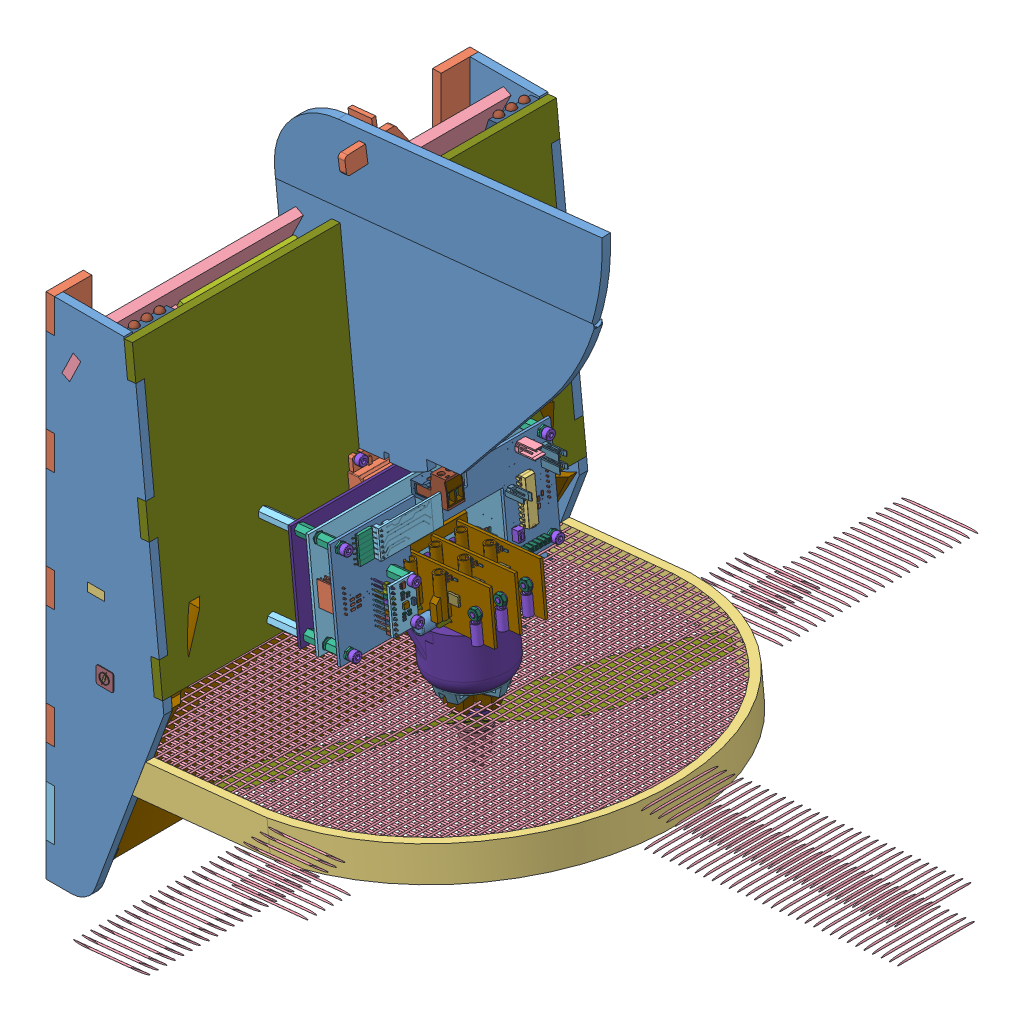
SolidWorks assembly AssTotale, configuration Défaut. Lengths in mm. (continued)
Components (placement in the parent): (continued)
- AssStructSimu-1: AssStructSimu [Défaut] at (-75.9431 -10.8604 24.5323) size (253.25 324.59 251.6) (continued)
  - AssCarte-1: AssCarte [Défaut] at (-42.8534 32.2132 302.028) x (-0.101852 0.9948 0) z (0.9948 0.101852 0) size (67.15 130.57 98.45) (continued)
    - carte_onduleur_v4-1: carte_onduleur_v4 [Défaut] at (-25.7639 0.8332 112.9379) size (66.52 130.57 82.34) (continued)
      - CON_IO1-1: CON_IO1 [Défaut] at (-11.3 12.1 0.803) x (0 -1 0) z (0 0 1) size (16.74 30.7 57.5) (continued)
        - Open CASCADE STEP translator 6.8 1.3.1-1: Open CASCADE STEP translator 6.8 1.3.1 [Défaut] at origin size (16.74 30.7 57.5) (continued)
          - Body_1_2-1: Body_1_2 [Défaut] at (-3 -15 8) x (0 -1 0) z (-1 0 0) size (30.7 57.5 16.74) (continued)
            - 57-1: 57 [Défaut] at (-15.3 2.7 -0.803) x (0 -1 0) z (0 0 -1) size (10.36 15.24 6.14) (continued)
              - =_[0_1_1_47]-1: =_[0_1_1_47] [Défaut] at origin size (10.36 15.24 6.14) (continued)
                - 55-1: 55 [Défaut] at (1.8 -1.2 3) x (1 0 0) z (0 1 0) size (10.36 6.14 15.24) (continued)
                  - 54-2: 54 [Défaut] at (0 0 -7.62) size (10.36 6.14 7.62) (continued)
                    - 52-2: 52 [Défaut] at (0 0 -2.54) size (10.36 6.14 2.54) (continued)
                      - 48-1: 48 [Défaut] at origin size (8.4 2.54 2.54)
                      - 49-1: 49 [Défaut] at (-0.0461 1.2682 1.27) x (0 0 -1) z (0.999998 -0.002105 0) size (1.95 5.07 7.58)
                    - 52-3: 52 [Défaut] at (0 0 -5.08) size (10.36 6.14 2.54)
                      - 48-1: 48 [Défaut] at origin size (8.4 2.54 2.54)
                      - 49-1: 49 [Défaut] at (-0.0461 1.2682 1.27) x (0 0 -1) z (0.999998 -0.002105 0) size (1.95 5.07 7.58)
            - 59-1: 59 [Défaut] at (-26.5 31 0.803) x (0 -1 0) z (0 0 1) size (2.34 1.04 0.5)
              - =_[0_1_1_42]-1: =_[0_1_1_42] [Défaut] at origin size (2.34 1.04 0.5)
                - 43-1: 43 [Défaut] at origin size (2.29 1.04 0.43)
                - 44-1: 44 [Défaut] at (0.3048 0 0) x (-1 0 0) z (0 0 1) size (0.51 1.02 0.5)
                - 45-1: 45 [Défaut] at origin size (0.51 1.02 0.5)
            - 61-1: 61 [Défaut] at (-21.6 17.8 0.803) x (-1 0 0) z (0 0 1) size (2.34 1.04 0.5)
              - =_[0_1_1_42]-1: =_[0_1_1_42] [Défaut] at origin size (2.34 1.04 0.5)
                - 43-1: 43 [Défaut] at origin size (2.29 1.04 0.43)
                - 44-1: 44 [Défaut] at (0.3048 0 0) x (-1 0 0) z (0 0 1) size (0.51 1.02 0.5)
                - 45-1: 45 [Défaut] at origin size (0.51 1.02 0.5)
            - 64-1: 64 [Défaut] at (-3.3 17.6 0.803) x (0 -1 0) z (0 0 1) size (8.01 8 14.24)
              - =_[0_1_1_56]-1: =_[0_1_1_56] [Défaut] at origin size (8.01 8 14.24)
                - 62-1: 62 [Défaut] at (1.8 0 0) x (1 0 0) z (0 -1 0) size (8.01 14.24 8)
      - CON_IO2-1: CON_IO2 [Défaut] at (-11.3 -2.7 0.803) x (0 -1 0) z (0 0 1) size (16.74 30.7 57.5)
        - Open CASCADE STEP translator 6.8 1.4.1-1: Open CASCADE STEP translator 6.8 1.4.1 [Défaut] at origin size (16.74 30.7 57.5)
          - Body_1_2-1: Body_1_2 [Défaut] at (-3 -15 8) x (0 -1 0) z (-1 0 0) size (30.7 57.5 16.74)
            - 1-1: 1 [Défaut] at origin size (30 50 1.61)
            - 10-1: 10 [Défaut] at (-14.395 31.0465 0.803) x (-1 0 0) z (0 0 1) size (5.59 6.35 1.11)
              - =_[0_1_1_4]-1: =_[0_1_1_4] [Défaut] at origin size (5.59 6.35 1.11)
                - 11-1: 11 [Défaut] at (2 3.3 0) x (-1 0 0) z (0 0 1) size (5.59 6.35 1.11)
                  - =_[0_1_1_3]_2-1: =_[0_1_1_3]_2 [Défaut] at origin size (0.44 0.55 0.36)
                  - =_[0_1_1_4]_2-1: =_[0_1_1_4]_2 [Défaut] at origin size (5.59 4.15 0.36)
                  - =_[0_1_1_5]_2-1: =_[0_1_1_5]_2 [Défaut] at origin size (5.35 6.1 1.1)
                  - =_[0_1_1_6]-1: =_[0_1_1_6] [Défaut] at origin size (0.44 0.55 0.36)
                  - =_[0_1_1_7]-1: =_[0_1_1_7] [Défaut] at origin size (0.44 0.55 0.36)
                  - =_[0_1_1_8]-1: =_[0_1_1_8] [Défaut] at origin size (0.44 0.55 0.36)
            - 13-1: 13 [Défaut] at (-12.62 16.6 -0.803) x (-1 0 0) z (0 0 -1) size (5.59 6.35 1.11)
              - =_[0_1_1_13]-1: =_[0_1_1_13] [Défaut] at origin size (5.59 6.35 1.11)
                - 11-1: 11 [Défaut] at (2 3.3 0) x (-1 0 0) z (0 0 1) size (5.59 6.35 1.11)
                  - =_[0_1_1_3]_2-1: =_[0_1_1_3]_2 [Défaut] at origin size (0.44 0.55 0.36)
                  - =_[0_1_1_4]_2-1: =_[0_1_1_4]_2 [Défaut] at origin size (5.59 4.15 0.36)
                  - =_[0_1_1_5]_2-1: =_[0_1_1_5]_2 [Défaut] at origin size (5.35 6.1 1.1)
                  - =_[0_1_1_6]-1: =_[0_1_1_6] [Défaut] at origin size (0.44 0.55 0.36)
                  - =_[0_1_1_7]-1: =_[0_1_1_7] [Défaut] at origin size (0.44 0.55 0.36)
                  - =_[0_1_1_8]-1: =_[0_1_1_8] [Défaut] at origin size (0.44 0.55 0.36)
            - 16-1: 16 [Défaut] at (-4.2 24.2 0.803) x (-1 0 0) z (0 0 1) size (12.8 0.5 13)
              - =_[0_1_1_15]-1: =_[0_1_1_15] [Défaut] at origin size (12.8 0.5 13)
                - 17-1: 17 [Défaut] at (2.7 0 0) x (1 0 0) z (0 -1 0) size (12.8 13 0.5)
            - 19-1: 19 [Défaut] at (-4.1 6.8 0.803) x (-1 0 0) z (0 0 1) size (12.8 0.5 13)
              - =_[0_1_1_18]-1: =_[0_1_1_18] [Défaut] at origin size (12.8 0.5 13)
                - 17-1: 17 [Défaut] at (2.7 0 0) x (1 0 0) z (0 -1 0) size (12.8 13 0.5)
            - 24-1: 24 [Défaut] at (-8.1 16.5 -0.803) x (0 1 0) z (0 0 -1) size (7.75 5.13 1.17)
              - =_[0_1_1_20]-1: =_[0_1_1_20] [Défaut] at origin size (7.75 5.13 1.17)
                - 20-1: 20 [Défaut] at origin size (7.59 5.13 1.07)
                - 21-1: 21 [Défaut] at (-14.478 0 0) x (-1 0 0) z (0 0 1) size (0.76 5.08 1.17)
                - 22-1: 22 [Défaut] at origin size (0.76 5.08 1.17)
            - 35-1: 35 [Défaut] at (-25.3 25.5 0.803) x (0 -1 0) z (0 0 1) size (6.05 5.2 1.7)
              - =_[0_1_1_25]-1: =_[0_1_1_25] [Défaut] at origin size (6.05 5.2 1.7)
                - 25-1: 25 [Défaut] at origin size (4.3 5.2 1.53)
                - 26-1: 26 [Défaut] at origin size (0.88 0.51 1.06)
                - 27-1: 27 [Défaut] at origin size (0.88 0.51 1.06)
                - 28-1: 28 [Défaut] at origin size (0.88 0.51 1.06)
                - 29-1: 29 [Défaut] at origin size (0.88 0.51 1.06)
                - 30-1: 30 [Défaut] at (11.6 -5.08 0) x (-1 0 0) z (0 0 1) size (0.87 0.51 1.06)
                - 31-1: 31 [Défaut] at (11.6 -2.54 0) x (-1 0 0) z (0 0 1) size (0.87 0.51 1.06)
                - 32-1: 32 [Défaut] at (11.6 0 0) x (-1 0 0) z (0 0 1) size (0.87 0.51 1.06)
                - 33-1: 33 [Défaut] at (11.6 2.54 0) x (-1 0 0) z (0 0 1) size (0.87 0.51 1.06)
            - 40-1: 40 [Défaut] at (-27.6 27.2 0.803) size (2.34 1.04 0.5)
              - =_[0_1_1_36]-1: =_[0_1_1_36] [Défaut] at origin size (2.34 1.04 0.5)
                - 36-1: 36 [Défaut] at origin size (2.29 1.04 0.43)
                - 37-1: 37 [Défaut] at (0.3048 0 0) x (-1 0 0) z (0 0 1) size (0.51 1.02 0.5)
                - 38-1: 38 [Défaut] at origin size (0.51 1.02 0.5)
            - 42-1: 42 [Défaut] at (-22.1 21.6 0.803) x (0 1 0) z (0 0 1) size (2.34 1.04 0.5)
              - =_[0_1_1_36]-1: =_[0_1_1_36] [Défaut] at origin size (2.34 1.04 0.5)
                - 36-1: 36 [Défaut] at origin size (2.29 1.04 0.43)
                - 37-1: 37 [Défaut] at (0.3048 0 0) x (-1 0 0) z (0 0 1) size (0.51 1.02 0.5)
                - 38-1: 38 [Défaut] at origin size (0.51 1.02 0.5)
            - 47-1: 47 [Défaut] at (-14.7664 14.5 -0.803) x (-1 0 0) z (0 0 -1) size (2.34 1.04 0.5)
              - =_[0_1_1_42]-1: =_[0_1_1_42] [Défaut] at origin size (2.34 1.04 0.5)
                - 43-1: 43 [Défaut] at origin size (2.29 1.04 0.43)
                - 44-1: 44 [Défaut] at (0.3048 0 0) x (-1 0 0) z (0 0 1) size (0.51 1.02 0.5)
                - 45-1: 45 [Défaut] at origin size (0.51 1.02 0.5)
            - 57-1: 57 [Défaut] at (-15.3 2.7 -0.803) x (0 -1 0) z (0 0 -1) size (10.36 15.24 6.14)
              - =_[0_1_1_47]-1: =_[0_1_1_47] [Défaut] at origin size (10.36 15.24 6.14)
                - 55-1: 55 [Défaut] at (1.8 -1.2 3) x (1 0 0) z (0 1 0) size (10.36 6.14 15.24)
                  - 54-1: 54 [Défaut] at origin size (10.36 6.14 7.62)
                    - 52-1: 52 [Défaut] at origin size (10.36 6.14 2.54)
                      - 48-1: 48 [Défaut] at origin size (8.4 2.54 2.54)
                      - 49-1: 49 [Défaut] at (-0.0461 1.2682 1.27) x (0 0 -1) z (0.999998 -0.002105 0) size (1.95 5.07 7.58)
                    - 52-2: 52 [Défaut] at (0 0 -2.54) size (10.36 6.14 2.54)
                      - 48-1: 48 [Défaut] at origin size (8.4 2.54 2.54)
                      - 49-1: 49 [Défaut] at (-0.0461 1.2682 1.27) x (0 0 -1) z (0.999998 -0.002105 0) size (1.95 5.07 7.58)
                    - 52-3: 52 [Défaut] at (0 0 -5.08) size (10.36 6.14 2.54)
                      - 48-1: 48 [Défaut] at origin size (8.4 2.54 2.54)
                      - 49-1: 49 [Défaut] at (-0.0461 1.2682 1.27) x (0 0 -1) z (0.999998 -0.002105 0) size (1.95 5.07 7.58)
                  - 54-2: 54 [Défaut] at (0 0 -7.62) size (10.36 6.14 7.62)
                    - 52-1: 52 [Défaut] at origin size (10.36 6.14 2.54)
                      - 48-1: 48 [Défaut] at origin size (8.4 2.54 2.54)
                      - 49-1: 49 [Défaut] at (-0.0461 1.2682 1.27) x (0 0 -1) z (0.999998 -0.002105 0) size (1.95 5.07 7.58)
                    - 52-2: 52 [Défaut] at (0 0 -2.54) size (10.36 6.14 2.54)
                      - 48-1: 48 [Défaut] at origin size (8.4 2.54 2.54)
                      - 49-1: 49 [Défaut] at (-0.0461 1.2682 1.27) x (0 0 -1) z (0.999998 -0.002105 0) size (1.95 5.07 7.58)
                    - 52-3: 52 [Défaut] at (0 0 -5.08) size (10.36 6.14 2.54)
                      - 48-1: 48 [Défaut] at origin size (8.4 2.54 2.54)
                      - 49-1: 49 [Défaut] at (-0.0461 1.2682 1.27) x (0 0 -1) z (0.999998 -0.002105 0) size (1.95 5.07 7.58)
            - 59-1: 59 [Défaut] at (-26.5 31 0.803) x (0 -1 0) z (0 0 1) size (2.34 1.04 0.5)
              - =_[0_1_1_42]-1: =_[0_1_1_42] [Défaut] at origin size (2.34 1.04 0.5)
                - 43-1: 43 [Défaut] at origin size (2.29 1.04 0.43)
                - 44-1: 44 [Défaut] at (0.3048 0 0) x (-1 0 0) z (0 0 1) size (0.51 1.02 0.5)
                - 45-1: 45 [Défaut] at origin size (0.51 1.02 0.5)
            - 61-1: 61 [Défaut] at (-21.6 17.8 0.803) x (-1 0 0) z (0 0 1) size (2.34 1.04 0.5)
              - =_[0_1_1_42]-1: =_[0_1_1_42] [Défaut] at origin size (2.34 1.04 0.5)
                - 43-1: 43 [Défaut] at origin size (2.29 1.04 0.43)
                - 44-1: 44 [Défaut] at (0.3048 0 0) x (-1 0 0) z (0 0 1) size (0.51 1.02 0.5)
                - 45-1: 45 [Défaut] at origin size (0.51 1.02 0.5)
            - 64-1: 64 [Défaut] at (-3.3 17.6 0.803) x (0 -1 0) z (0 0 1) size (8.01 8 14.24)
              - =_[0_1_1_56]-1: =_[0_1_1_56] [Défaut] at origin size (8.01 8 14.24)
                - 62-1: 62 [Défaut] at (1.8 0 0) x (1 0 0) z (0 -1 0) size (8.01 14.24 8)
      - CON_IO3-1: CON_IO3 [Défaut] at (-11.3 -17.7 0.803) x (0 -1 0) z (0 0 1) size (16.74 30.7 57.5)
        - Open CASCADE STEP translator 6.8 1.5.1-1: Open CASCADE STEP translator 6.8 1.5.1 [Défaut] at origin size (16.74 30.7 57.5)
          - Body_1_2-1: Body_1_2 [Défaut] at (-3 -15 8) x (0 -1 0) z (-1 0 0) size (30.7 57.5 16.74)
            - 1-1: 1 [Défaut] at origin size (30 50 1.61)
            - 10-1: 10 [Défaut] at (-14.395 31.0465 0.803) x (-1 0 0) z (0 0 1) size (5.59 6.35 1.11)
              - =_[0_1_1_4]-1: =_[0_1_1_4] [Défaut] at origin size (5.59 6.35 1.11)
                - 11-1: 11 [Défaut] at (2 3.3 0) x (-1 0 0) z (0 0 1) size (5.59 6.35 1.11)
                  - =_[0_1_1_3]_2-1: =_[0_1_1_3]_2 [Défaut] at origin size (0.44 0.55 0.36)
                  - =_[0_1_1_4]_2-1: =_[0_1_1_4]_2 [Défaut] at origin size (5.59 4.15 0.36)
                  - =_[0_1_1_5]_2-1: =_[0_1_1_5]_2 [Défaut] at origin size (5.35 6.1 1.1)
                  - =_[0_1_1_6]-1: =_[0_1_1_6] [Défaut] at origin size (0.44 0.55 0.36)
                  - =_[0_1_1_7]-1: =_[0_1_1_7] [Défaut] at origin size (0.44 0.55 0.36)
                  - =_[0_1_1_8]-1: =_[0_1_1_8] [Défaut] at origin size (0.44 0.55 0.36)
            - 13-1: 13 [Défaut] at (-12.62 16.6 -0.803) x (-1 0 0) z (0 0 -1) size (5.59 6.35 1.11)
              - =_[0_1_1_13]-1: =_[0_1_1_13] [Défaut] at origin size (5.59 6.35 1.11)
                - 11-1: 11 [Défaut] at (2 3.3 0) x (-1 0 0) z (0 0 1) size (5.59 6.35 1.11)
                  - =_[0_1_1_3]_2-1: =_[0_1_1_3]_2 [Défaut] at origin size (0.44 0.55 0.36)
                  - =_[0_1_1_4]_2-1: =_[0_1_1_4]_2 [Défaut] at origin size (5.59 4.15 0.36)
                  - =_[0_1_1_5]_2-1: =_[0_1_1_5]_2 [Défaut] at origin size (5.35 6.1 1.1)
                  - =_[0_1_1_6]-1: =_[0_1_1_6] [Défaut] at origin size (0.44 0.55 0.36)
                  - =_[0_1_1_7]-1: =_[0_1_1_7] [Défaut] at origin size (0.44 0.55 0.36)
                  - =_[0_1_1_8]-1: =_[0_1_1_8] [Défaut] at origin size (0.44 0.55 0.36)
            - 16-1: 16 [Défaut] at (-4.2 24.2 0.803) x (-1 0 0) z (0 0 1) size (12.8 0.5 13)
              - =_[0_1_1_15]-1: =_[0_1_1_15] [Défaut] at origin size (12.8 0.5 13)
                - 17-1: 17 [Défaut] at (2.7 0 0) x (1 0 0) z (0 -1 0) size (12.8 13 0.5)
            - 19-1: 19 [Défaut] at (-4.1 6.8 0.803) x (-1 0 0) z (0 0 1) size (12.8 0.5 13)
              - =_[0_1_1_18]-1: =_[0_1_1_18] [Défaut] at origin size (12.8 0.5 13)
                - 17-1: 17 [Défaut] at (2.7 0 0) x (1 0 0) z (0 -1 0) size (12.8 13 0.5)
            - 24-1: 24 [Défaut] at (-8.1 16.5 -0.803) x (0 1 0) z (0 0 -1) size (7.75 5.13 1.17)
              - =_[0_1_1_20]-1: =_[0_1_1_20] [Défaut] at origin size (7.75 5.13 1.17)
                - 20-1: 20 [Défaut] at origin size (7.59 5.13 1.07)
                - 21-1: 21 [Défaut] at (-14.478 0 0) x (-1 0 0) z (0 0 1) size (0.76 5.08 1.17)
                - 22-1: 22 [Défaut] at origin size (0.76 5.08 1.17)
            - 35-1: 35 [Défaut] at (-25.3 25.5 0.803) x (0 -1 0) z (0 0 1) size (6.05 5.2 1.7)
              - =_[0_1_1_25]-1: =_[0_1_1_25] [Défaut] at origin size (6.05 5.2 1.7)
                - 25-1: 25 [Défaut] at origin size (4.3 5.2 1.53)
                - 26-1: 26 [Défaut] at origin size (0.88 0.51 1.06)
                - 27-1: 27 [Défaut] at origin size (0.88 0.51 1.06)
                - 28-1: 28 [Défaut] at origin size (0.88 0.51 1.06)
                - 29-1: 29 [Défaut] at origin size (0.88 0.51 1.06)
                - 30-1: 30 [Défaut] at (11.6 -5.08 0) x (-1 0 0) z (0 0 1) size (0.87 0.51 1.06)
                - 31-1: 31 [Défaut] at (11.6 -2.54 0) x (-1 0 0) z (0 0 1) size (0.87 0.51 1.06)
                - 32-1: 32 [Défaut] at (11.6 0 0) x (-1 0 0) z (0 0 1) size (0.87 0.51 1.06)
                - 33-1: 33 [Défaut] at (11.6 2.54 0) x (-1 0 0) z (0 0 1) size (0.87 0.51 1.06)
            - 40-1: 40 [Défaut] at (-27.6 27.2 0.803) size (2.34 1.04 0.5)
              - =_[0_1_1_36]-1: =_[0_1_1_36] [Défaut] at origin size (2.34 1.04 0.5)
                - 36-1: 36 [Défaut] at origin size (2.29 1.04 0.43)
                - 37-1: 37 [Défaut] at (0.3048 0 0) x (-1 0 0) z (0 0 1) size (0.51 1.02 0.5)
                - 38-1: 38 [Défaut] at origin size (0.51 1.02 0.5)
            - 42-1: 42 [Défaut] at (-22.1 21.6 0.803) x (0 1 0) z (0 0 1) size (2.34 1.04 0.5)
              - =_[0_1_1_36]-1: =_[0_1_1_36] [Défaut] at origin size (2.34 1.04 0.5)
                - 36-1: 36 [Défaut] at origin size (2.29 1.04 0.43)
                - 37-1: 37 [Défaut] at (0.3048 0 0) x (-1 0 0) z (0 0 1) size (0.51 1.02 0.5)
                - 38-1: 38 [Défaut] at origin size (0.51 1.02 0.5)
            - 47-1: 47 [Défaut] at (-14.7664 14.5 -0.803) x (-1 0 0) z (0 0 -1) size (2.34 1.04 0.5)
              - =_[0_1_1_42]-1: =_[0_1_1_42] [Défaut] at origin size (2.34 1.04 0.5)
                - 43-1: 43 [Défaut] at origin size (2.29 1.04 0.43)
                - 44-1: 44 [Défaut] at (0.3048 0 0) x (-1 0 0) z (0 0 1) size (0.51 1.02 0.5)
                - 45-1: 45 [Défaut] at origin size (0.51 1.02 0.5)
            - 57-1: 57 [Défaut] at (-15.3 2.7 -0.803) x (0 -1 0) z (0 0 -1) size (10.36 15.24 6.14)
              - =_[0_1_1_47]-1: =_[0_1_1_47] [Défaut] at origin size (10.36 15.24 6.14)
                - 55-1: 55 [Défaut] at (1.8 -1.2 3) x (1 0 0) z (0 1 0) size (10.36 6.14 15.24)
                  - 54-1: 54 [Défaut] at origin size (10.36 6.14 7.62)
                    - 52-1: 52 [Défaut] at origin size (10.36 6.14 2.54)
                      - 48-1: 48 [Défaut] at origin size (8.4 2.54 2.54)
                      - 49-1: 49 [Défaut] at (-0.0461 1.2682 1.27) x (0 0 -1) z (0.999998 -0.002105 0) size (1.95 5.07 7.58)
                    - 52-2: 52 [Défaut] at (0 0 -2.54) size (10.36 6.14 2.54)
                      - 48-1: 48 [Défaut] at origin size (8.4 2.54 2.54)
                      - 49-1: 49 [Défaut] at (-0.0461 1.2682 1.27) x (0 0 -1) z (0.999998 -0.002105 0) size (1.95 5.07 7.58)
                    - 52-3: 52 [Défaut] at (0 0 -5.08) size (10.36 6.14 2.54)
                      - 48-1: 48 [Défaut] at origin size (8.4 2.54 2.54)
                      - 49-1: 49 [Défaut] at (-0.0461 1.2682 1.27) x (0 0 -1) z (0.999998 -0.002105 0) size (1.95 5.07 7.58)
                  - 54-2: 54 [Défaut] at (0 0 -7.62) size (10.36 6.14 7.62)
                    - 52-1: 52 [Défaut] at origin size (10.36 6.14 2.54)
                      - 48-1: 48 [Défaut] at origin size (8.4 2.54 2.54)
                      - 49-1: 49 [Défaut] at (-0.0461 1.2682 1.27) x (0 0 -1) z (0.999998 -0.002105 0) size (1.95 5.07 7.58)
                    - 52-2: 52 [Défaut] at (0 0 -2.54) size (10.36 6.14 2.54)
                      - 48-1: 48 [Défaut] at origin size (8.4 2.54 2.54)
                      - 49-1: 49 [Défaut] at (-0.0461 1.2682 1.27) x (0 0 -1) z (0.999998 -0.002105 0) size (1.95 5.07 7.58)
                    - 52-3: 52 [Défaut] at (0 0 -5.08) size (10.36 6.14 2.54)
                      - 48-1: 48 [Défaut] at origin size (8.4 2.54 2.54)
                      - 49-1: 49 [Défaut] at (-0.0461 1.2682 1.27) x (0 0 -1) z (0.999998 -0.002105 0) size (1.95 5.07 7.58)
            - 59-1: 59 [Défaut] at (-26.5 31 0.803) x (0 -1 0) z (0 0 1) size (2.34 1.04 0.5)
              - =_[0_1_1_42]-1: =_[0_1_1_42] [Défaut] at origin size (2.34 1.04 0.5)
                - 43-1: 43 [Défaut] at origin size (2.29 1.04 0.43)
                - 44-1: 44 [Défaut] at (0.3048 0 0) x (-1 0 0) z (0 0 1) size (0.51 1.02 0.5)
                - 45-1: 45 [Défaut] at origin size (0.51 1.02 0.5)
            - 61-1: 61 [Défaut] at (-21.6 17.8 0.803) x (-1 0 0) z (0 0 1) size (2.34 1.04 0.5)
              - =_[0_1_1_42]-1: =_[0_1_1_42] [Défaut] at origin size (2.34 1.04 0.5)
                - 43-1: 43 [Défaut] at origin size (2.29 1.04 0.43)
                - 44-1: 44 [Défaut] at (0.3048 0 0) x (-1 0 0) z (0 0 1) size (0.51 1.02 0.5)
                - 45-1: 45 [Défaut] at origin size (0.51 1.02 0.5)
            - 64-1: 64 [Défaut] at (-3.3 17.6 0.803) x (0 -1 0) z (0 0 1) size (8.01 8 14.24)
              - =_[0_1_1_56]-1: =_[0_1_1_56] [Défaut] at origin size (8.01 8 14.24)
                - 62-1: 62 [Défaut] at (1.8 0 0) x (1 0 0) z (0 -1 0) size (8.01 14.24 8)
      - C1_1-1: C1_1 [Défaut] at (-20.6336 6.4 -0.803) x (1 0 0) z (0 0 -1) size (2.34 1.04 0.5)
        - Open CASCADE STEP translator 6.8 1.6.1-1: Open CASCADE STEP translator 6.8 1.6.1 [Défaut] at origin size (2.34 1.04 0.5)
          - Body_1-1: Body_1 [Défaut] at origin size (2.29 1.04 0.43)
          - Pin_1-1: Pin_1 [Défaut] at (0.3048 0 0) x (-1 0 0) z (0 0 1) size (0.51 1.02 0.5)
          - Pin_2-1: Pin_2 [Défaut] at origin size (0.51 1.02 0.5)
      - C1_2-1: C1_2 [Défaut] at (-24.2 6.4 -0.803) x (1 0 0) z (0 0 -1) size (2.34 1.04 0.5)
        - Open CASCADE STEP translator 6.8 1.6.1-1: Open CASCADE STEP translator 6.8 1.6.1 [Défaut] at origin size (2.34 1.04 0.5)
          - Body_1-1: Body_1 [Défaut] at origin size (2.29 1.04 0.43)
          - Pin_1-1: Pin_1 [Défaut] at (0.3048 0 0) x (-1 0 0) z (0 0 1) size (0.51 1.02 0.5)
          - Pin_2-1: Pin_2 [Défaut] at origin size (0.51 1.02 0.5)
      - C_F-1: C_F [Défaut] at (-16.2432 4.45 -0.803) x (0 -1 0) z (0 0 -1) size (2.34 1.04 0.5)
        - Open CASCADE STEP translator 6.8 1.6.1-1: Open CASCADE STEP translator 6.8 1.6.1 [Défaut] at origin size (2.34 1.04 0.5)
          - Body_1-1: Body_1 [Défaut] at origin size (2.29 1.04 0.43)
          - Pin_1-1: Pin_1 [Défaut] at (0.3048 0 0) x (-1 0 0) z (0 0 1) size (0.51 1.02 0.5)
          - Pin_2-1: Pin_2 [Défaut] at origin size (0.51 1.02 0.5)
      - D_LED_STATE1-1: D_LED_STATE1 [Défaut] at (-6.8906 -21.6 0.803) size (2.34 1.04 0.5)
        - Open CASCADE STEP translator 6.8 1.6.1-1: Open CASCADE STEP translator 6.8 1.6.1 [Défaut] at origin size (2.34 1.04 0.5)
          - Body_1-1: Body_1 [Défaut] at origin size (2.29 1.04 0.43)
          - Pin_1-1: Pin_1 [Défaut] at (0.3048 0 0) x (-1 0 0) z (0 0 1) size (0.51 1.02 0.5)
          - Pin_2-1: Pin_2 [Défaut] at origin size (0.51 1.02 0.5)
      - PICKIT-1: PICKIT [Défaut] at (-24.1 -30.5 0.803) size (15.24 5 14.3)
        - Open CASCADE STEP translator 6.8 1.10.1-1: Open CASCADE STEP translator 6.8 1.10.1 [Défaut] at origin size (15.24 5 14.3)
          - Body_1_2-1: Body_1_2 [Défaut] at (6.3 0 12) size (15.24 5 14.3)
      - C_DEC_CUR-1: C_DEC_CUR [Défaut] at (-8.9496 5.7572 -0.803) x (0 1 0) z (0 0 -1) size (2.34 1.04 0.5)
        - Open CASCADE STEP translator 6.8 1.6.1-1: Open CASCADE STEP translator 6.8 1.6.1 [Défaut] at origin size (2.34 1.04 0.5)
          - Body_1-1: Body_1 [Défaut] at origin size (2.29 1.04 0.43)
          - Pin_1-1: Pin_1 [Défaut] at (0.3048 0 0) x (-1 0 0) z (0 0 1) size (0.51 1.02 0.5)
          - Pin_2-1: Pin_2 [Défaut] at origin size (0.51 1.02 0.5)
      - R_F-1: R_F [Défaut] at (-14.65 4.4432 -0.803) x (0 -1 0) z (0 0 -1) size (2.34 1.04 0.5)
        - Open CASCADE STEP translator 6.8 1.12.1-1: Open CASCADE STEP translator 6.8 1.12.1 [Défaut] at origin size (2.34 1.04 0.5)
          - Body_1_3-1: Body_1_3 [Défaut] at origin size (2.29 1.04 0.43)
          - Pin_1_2-1: Pin_1_2 [Défaut] at (0.3048 0 0) x (-1 0 0) z (0 0 1) size (0.51 1.02 0.5)
          - Pin_2_2-1: Pin_2_2 [Défaut] at origin size (0.51 1.02 0.5)
      - R_GAIN1-1: R_GAIN1 [Défaut] at (-13.95 5.7568 -0.803) x (0 1 0) z (0 0 -1) size (2.34 1.04 0.5)
        - Open CASCADE STEP translator 6.8 1.12.1-1: Open CASCADE STEP translator 6.8 1.12.1 [Défaut] at origin size (2.34 1.04 0.5)
          - Body_1_3-1: Body_1_3 [Défaut] at origin size (2.29 1.04 0.43)
          - Pin_1_2-1: Pin_1_2 [Défaut] at (0.3048 0 0) x (-1 0 0) z (0 0 1) size (0.51 1.02 0.5)
          - Pin_2_2-1: Pin_2_2 [Défaut] at origin size (0.51 1.02 0.5)
      - R_GAIN2-1: R_GAIN2 [Défaut] at (-15.65 7.9176 -0.803) x (0 -1 0) z (0 0 -1) size (2.34 1.04 0.5)
        - Open CASCADE STEP translator 6.8 1.12.1-1: Open CASCADE STEP translator 6.8 1.12.1 [Défaut] at origin size (2.34 1.04 0.5)
          - Body_1_3-1: Body_1_3 [Défaut] at origin size (2.29 1.04 0.43)
          - Pin_1_2-1: Pin_1_2 [Défaut] at (0.3048 0 0) x (-1 0 0) z (0 0 1) size (0.51 1.02 0.5)
          - Pin_2_2-1: Pin_2_2 [Défaut] at origin size (0.51 1.02 0.5)
      - R_LED_STATE1-1: R_LED_STATE1 [Défaut] at (-6.9242 -19.9 0.803) size (2.34 1.04 0.5)
        - Open CASCADE STEP translator 6.8 1.12.1-1: Open CASCADE STEP translator 6.8 1.12.1 [Défaut] at origin size (2.34 1.04 0.5)
          - Body_1_3-1: Body_1_3 [Défaut] at origin size (2.29 1.04 0.43)
          - Pin_1_2-1: Pin_1_2 [Défaut] at (0.3048 0 0) x (-1 0 0) z (0 0 1) size (0.51 1.02 0.5)
          - Pin_2_2-1: Pin_2_2 [Défaut] at origin size (0.51 1.02 0.5)
      - R_RESET1-1: R_RESET1 [Défaut] at (-23 7.9 0.803) size (2.34 1.04 0.5)
        - Open CASCADE STEP translator 6.8 1.12.1-1: Open CASCADE STEP translator 6.8 1.12.1 [Défaut] at origin size (2.34 1.04 0.5)
          - Body_1_3-1: Body_1_3 [Défaut] at origin size (2.29 1.04 0.43)
          - Pin_1_2-1: Pin_1_2 [Défaut] at (0.3048 0 0) x (-1 0 0) z (0 0 1) size (0.51 1.02 0.5)
          - Pin_2_2-1: Pin_2_2 [Défaut] at origin size (0.51 1.02 0.5)
      - U_DSPIC-1: U_DSPIC [Défaut] at (1.863 -2.61 0.803) size (7.92 35.56 7.75)
        - Open CASCADE STEP translator 6.8 1.17.1-1: Open CASCADE STEP translator 6.8 1.17.1 [Défaut] at origin size (7.92 35.56 7.75)
          - Body_1_4-1: Body_1_4 [Défaut] at (0 -0.2 4) x (1 0 0) z (0 -1 0) size (7.92 7.75 35.56)
      - C_DEC_DSPIC-1: C_DEC_DSPIC [Défaut] at (7.7 -8.8 -0.803) x (0 1 0) z (0 0 -1) size (2.34 1.04 0.5)
        - Open CASCADE STEP translator 6.8 1.6.1-1: Open CASCADE STEP translator 6.8 1.6.1 [Défaut] at origin size (2.34 1.04 0.5)
          - Body_1-1: Body_1 [Défaut] at origin size (2.29 1.04 0.43)
          - Pin_1-1: Pin_1 [Défaut] at (0.3048 0 0) x (-1 0 0) z (0 0 1) size (0.51 1.02 0.5)
          - Pin_2-1: Pin_2 [Défaut] at origin size (0.51 1.02 0.5)
      - IN-1: IN [Défaut] at (24.3 -5.3 0.803) x (0 1 0) z (0 0 1) size (10.21 15.56 26.9)
        - Open CASCADE STEP translator 6.8 1.19.1-1: Open CASCADE STEP translator 6.8 1.19.1 [Défaut] at origin size (10.21 15.56 26.9)
          - Body_1_3-1: Body_1_3 [Défaut] at (-13.5 1.8 3) x (0 1 0) z (1 0 0) size (15.56 26.9 10.21)
            - Imported-1: Imported [Défaut] at (2.0451 -4.5908 20.9802) size (8.6 15.9 10.16)
            - Imported-2: Imported [Défaut] at (-1.6683 9.1092 15.9802) x (0 0 1) z (-1 0 0) size (10.1 18.2 15.1)
              - Imported_2-1: Imported_2 [Défaut] at origin size (10.1 18.2 15.1)
              - Imported_3-1: Imported_3 [Défaut] at origin size (3.43 12.4 4.99)
              - Imported_4-1: Imported_4 [Défaut] at origin size (3.43 12.4 4.99)
              - Imported_5-1: Imported_5 [Défaut] at origin size (3.9 4.9 7)
              - Imported_6-1: Imported_6 [Défaut] at origin size (3.9 4.9 7)
              - Imported_7-1: Imported_7 [Défaut] at origin size (3.8 3.8 6.92)
              - Imported_8-1: Imported_8 [Défaut] at origin size (3.8 3.8 6.92)
              - Imported_9-1: Imported_9 [Défaut] at origin size (9 2.4 14.2)
      - CARTE_CMD-1: CARTE_CMD [Défaut] at (25 57.2 0.803) size (60.1 130 26.71)
        - Open CASCADE STEP translator 6.8 1.20.1-1: Open CASCADE STEP translator 6.8 1.20.1 [Défaut] at origin size (60.1 130 26.71)
          - Body_1_4-1: Body_1_4 [Défaut] at (-55 5 12) size (60.1 130 26.71)
            - 1_2-1: 1_2 [Défaut] at origin size (60.1 130 1.61)
            - 4-1: 4 [Défaut] at (23.6 -124.9 0.803) x (0 1 0) z (0 0 1) size (5 15.24 14.3)
              - =_[0_1_1_4]_2-1: =_[0_1_1_4]_2 [Défaut] at origin size (5 15.24 14.3)
                - 5-1: 5 [Défaut] at (0 -6.5 -13) x (0 1 0) z (0 0 -1) size (15.24 5 14.3)
            - 7-1: 7 [Défaut] at (23.6 -5 0.803) x (0 1 0) z (0 0 1) size (5 15.24 14.3)
              - =_[0_1_1_7]-1: =_[0_1_1_7] [Défaut] at origin size (5 15.24 14.3)
                - 5-1: 5 [Défaut] at (0 -6.5 -13) x (0 1 0) z (0 0 -1) size (15.24 5 14.3)
            - 10_2-1: 10_2 [Défaut] at (18.4 -115.6 0.803) size (25.4 7.92 7.75)
              - =_[0_1_1_9]-1: =_[0_1_1_9] [Défaut] at origin size (25.4 7.92 7.75)
                - 8-1: 8 [Défaut] at (11.2 4 0) x (0 1 0) z (1 0 0) size (7.92 7.75 25.4)
            - 13_2-1: 13_2 [Défaut] at (55.4 -114.7 0.803) x (-1 0 0) z (0 0 1) size (5 7.62 14.3)
              - =_[0_1_1_12]-1: =_[0_1_1_12] [Défaut] at origin size (5 7.62 14.3)
                - 11-1: 11 [Défaut] at (0 -2.5 11) x (0 -1 0) z (0 0 1) size (7.62 5 14.3)
            - 25-1: 25 [Défaut] at (56.9 -12.8 0.803) x (-1 0 0) z (0 0 1) size (16.02 47.26 11.05)
              - =_[0_1_1_15]_2-1: =_[0_1_1_15]_2 [Défaut] at origin size (16.02 47.26 11.05)
                - 23-1: 23 [Défaut] at (-36.5 21 4) x (0 -1 0) z (1 0 0) size (47.26 11.05 16.02)
                  - 14-1: 14 [Défaut] at (-7.4961 -1.5352 42.5833) size (42.58 6.55 16.01)
                  - 22-1: 22 [Défaut] at (19.3039 2.3748 37.905) x (-1 0 0) z (0 0 -1) size (10.36 6.14 15.24)
                    - 21-1: 21 [Défaut] at origin size (10.36 6.14 7.62)
                      - 19_2-1: 19_2 [Défaut] at origin size (10.36 6.14 2.54)
                        - 15-1: 15 [Défaut] at origin size (8.4 2.54 2.54)
                        - 16-1: 16 [Défaut] at (-0.0461 1.2682 1.27) x (0 0 -1) z (0.999998 -0.002105 0) size (1.95 5.07 7.58)
                      - 19_2-2: 19_2 [Défaut] at (0 0 -2.54) size (10.36 6.14 2.54)
                        - 15-1: 15 [Défaut] at origin size (8.4 2.54 2.54)
                        - 16-1: 16 [Défaut] at (-0.0461 1.2682 1.27) x (0 0 -1) z (0.999998 -0.002105 0) size (1.95 5.07 7.58)
                      - 19_2-3: 19_2 [Défaut] at (0 0 -5.08) size (10.36 6.14 2.54)
                        - 15-1: 15 [Défaut] at origin size (8.4 2.54 2.54)
                        - 16-1: 16 [Défaut] at (-0.0461 1.2682 1.27) x (0 0 -1) z (0.999998 -0.002105 0) size (1.95 5.07 7.58)
                    - 21-2: 21 [Défaut] at (0 0 -7.62) size (10.36 6.14 7.62)
                      - 19_2-1: 19_2 [Défaut] at origin size (10.36 6.14 2.54)
                        - 15-1: 15 [Défaut] at origin size (8.4 2.54 2.54)
                        - 16-1: 16 [Défaut] at (-0.0461 1.2682 1.27) x (0 0 -1) z (0.999998 -0.002105 0) size (1.95 5.07 7.58)
                      - 19_2-2: 19_2 [Défaut] at (0 0 -2.54) size (10.36 6.14 2.54)
                        - 15-1: 15 [Défaut] at origin size (8.4 2.54 2.54)
                        - 16-1: 16 [Défaut] at (-0.0461 1.2682 1.27) x (0 0 -1) z (0.999998 -0.002105 0) size (1.95 5.07 7.58)
                      - 19_2-3: 19_2 [Défaut] at (0 0 -5.08) size (10.36 6.14 2.54)
                        - 15-1: 15 [Défaut] at origin size (8.4 2.54 2.54)
                        - 16-1: 16 [Défaut] at (-0.0461 1.2682 1.27) x (0 0 -1) z (0.999998 -0.002105 0) size (1.95 5.07 7.58)
            - 31-1: 31 [Défaut] at (12.9 -104.5 0.803) size (6.76 3.64 4.37)
              - =_[0_1_1_24]-1: =_[0_1_1_24] [Défaut] at origin size (6.76 3.64 4.37)
                - 29-1: 29 [Défaut] at (-0.3 -2 0) size (6.76 3.64 4.37)
                  - =_[0_1_1_3]_3-1: =_[0_1_1_3]_3 [Défaut] at origin size (6 3.64 4.37)
                  - =_[0_1_1_4]_3-1: =_[0_1_1_4]_3 [Défaut] at origin size (0.38 1 0.67)
                  - =_[0_1_1_5]_3-1: =_[0_1_1_5]_3 [Défaut] at origin size (0.38 1 0.67)
            - 36-1: 36 [Défaut] at (28.6 -12.2 0.803) x (0 -1 0) z (0 0 1) size (2.34 1.04 0.5)
              - =_[0_1_1_30]-1: =_[0_1_1_30] [Défaut] at origin size (2.34 1.04 0.5)
                - 32_2-1: 32_2 [Défaut] at origin size (2.29 1.04 0.43)
                - 33_2-1: 33_2 [Défaut] at (0.3048 0 0) x (-1 0 0) z (0 0 1) size (0.51 1.02 0.5)
                - 34-1: 34 [Défaut] at origin size (0.51 1.02 0.5)
            - 38-1: 38 [Défaut] at (23.7 -12.2 0.803) x (0 -1 0) z (0 0 1) size (2.34 1.04 0.5)
              - =_[0_1_1_30]-1: =_[0_1_1_30] [Défaut] at origin size (2.34 1.04 0.5)
                - 32_2-1: 32_2 [Défaut] at origin size (2.29 1.04 0.43)
                - 33_2-1: 33_2 [Défaut] at (0.3048 0 0) x (-1 0 0) z (0 0 1) size (0.51 1.02 0.5)
                - 34-1: 34 [Défaut] at origin size (0.51 1.02 0.5)
            - 40_2-1: 40_2 [Défaut] at (26.2 -12.2 0.803) x (0 -1 0) z (0 0 1) size (2.34 1.04 0.5)
              - =_[0_1_1_30]-1: =_[0_1_1_30] [Défaut] at origin size (2.34 1.04 0.5)
                - 32_2-1: 32_2 [Défaut] at origin size (2.29 1.04 0.43)
                - 33_2-1: 33_2 [Défaut] at (0.3048 0 0) x (-1 0 0) z (0 0 1) size (0.51 1.02 0.5)
                - 34-1: 34 [Défaut] at origin size (0.51 1.02 0.5)
            - 42_2-1: 42_2 [Défaut] at (24.4 -119.2 0.803) size (2.34 1.04 0.5)
              - =_[0_1_1_30]-1: =_[0_1_1_30] [Défaut] at origin size (2.34 1.04 0.5)
                - 32_2-1: 32_2 [Défaut] at origin size (2.29 1.04 0.43)
                - 33_2-1: 33_2 [Défaut] at (0.3048 0 0) x (-1 0 0) z (0 0 1) size (0.51 1.02 0.5)
                - 34-1: 34 [Défaut] at origin size (0.51 1.02 0.5)
            - 45-1: 45 [Défaut] at (46.4 -125 0.803) size (5.08 5 14.3)
              - =_[0_1_1_38]-1: =_[0_1_1_38] [Défaut] at origin size (5.08 5 14.3)
                - 190-1: 190 [Défaut] at (1.2 0 11) size (5.08 5 14.3)
            - 48-1: 48 [Défaut] at (40.1 -125 0.803) size (5.08 5 14.3)
              - =_[0_1_1_41]-1: =_[0_1_1_41] [Défaut] at origin size (5.08 5 14.3)
                - 190-1: 190 [Défaut] at (1.2 0 11) size (5.08 5 14.3)
            - 51-1: 51 [Défaut] at (6.4 -119.9 0.803) x (0 1 0) z (0 0 1) size (15.24 2.54 7.37)
              - =_[0_1_1_43]-1: =_[0_1_1_43] [Défaut] at origin size (15.24 2.54 7.37)
                - 49_2-1: 49_2 [Défaut] at (6.5 0 0) x (1 0 0) z (0 -1 0) size (15.24 7.37 2.54)
            - 57_2-1: 57_2 [Défaut] at (50.8796 -121.1 -0.803) x (-1 0 0) z (0 0 -1) size (2.54 1.98 0.64)
              - =_[0_1_1_46]-1: =_[0_1_1_46] [Défaut] at origin size (2.54 1.98 0.64)
                - 52-1: 52 [Défaut] at origin size (2.54 1.14 0.58)
                - 53-1: 53 [Défaut] x (0 -1 0) z (0 0 1) size (0.43 0.51 0.38)
                - 54-1: 54 [Défaut] at (1.8796 1.8796 0) x (0 -1 0) z (0 0 1) size (0.43 0.51 0.38)
                - 55-1: 55 [Défaut] at (-0.9652 -2.8448 0) x (0 1 0) z (0 0 1) size (0.41 0.51 0.38)
            - 59_2-1: 59_2 [Défaut] at (43.6398 -120.995 -0.803) x (-1 0 0) z (0 0 -1) size (2.54 1.98 0.64)
              - =_[0_1_1_46]-1: =_[0_1_1_46] [Défaut] at origin size (2.54 1.98 0.64)
                - 52-1: 52 [Défaut] at origin size (2.54 1.14 0.58)
                - 53-1: 53 [Défaut] x (0 -1 0) z (0 0 1) size (0.43 0.51 0.38)
                - 54-1: 54 [Défaut] at (1.8796 1.8796 0) x (0 -1 0) z (0 0 1) size (0.43 0.51 0.38)
                - 55-1: 55 [Défaut] at (-0.9652 -2.8448 0) x (0 1 0) z (0 0 1) size (0.41 0.51 0.38)
            - 61_2-1: 61_2 [Défaut] at (47.6 -119.9 -0.803) x (-1 0 0) z (0 0 -1) size (2.34 1.04 0.5)
              - =_[0_1_1_30]-1: =_[0_1_1_30] [Défaut] at origin size (2.34 1.04 0.5)
                - 32_2-1: 32_2 [Défaut] at origin size (2.29 1.04 0.43)
                - 33_2-1: 33_2 [Défaut] at (0.3048 0 0) x (-1 0 0) z (0 0 1) size (0.51 1.02 0.5)
                - 34-1: 34 [Défaut] at origin size (0.51 1.02 0.5)
            - 63-1: 63 [Défaut] at (40.4 -119.9 -0.803) x (-1 0 0) z (0 0 -1) size (2.34 1.04 0.5)
              - =_[0_1_1_30]-1: =_[0_1_1_30] [Défaut] at origin size (2.34 1.04 0.5)
                - 32_2-1: 32_2 [Défaut] at origin size (2.29 1.04 0.43)
                - 33_2-1: 33_2 [Défaut] at (0.3048 0 0) x (-1 0 0) z (0 0 1) size (0.51 1.02 0.5)
                - 34-1: 34 [Défaut] at origin size (0.51 1.02 0.5)
            - 68-1: 68 [Défaut] at (47.7 -21.8 -0.803) x (0 1 0) z (0 0 -1) size (2.34 1.04 0.5)
              - =_[0_1_1_55]-1: =_[0_1_1_55] [Défaut] at origin size (2.34 1.04 0.5)
                - 64-1: 64 [Défaut] at origin size (2.29 1.04 0.43)
                - 65-1: 65 [Défaut] at (0.3048 0 0) x (-1 0 0) z (0 0 1) size (0.51 1.02 0.5)
                - 66-1: 66 [Défaut] at origin size (0.51 1.02 0.5)
            - 70-1: 70 [Défaut] at (47.6 -121.7 -0.803) x (-1 0 0) z (0 0 -1) size (2.34 1.04 0.5)
              - =_[0_1_1_30]-1: =_[0_1_1_30] [Défaut] at origin size (2.34 1.04 0.5)
                - 32_2-1: 32_2 [Défaut] at origin size (2.29 1.04 0.43)
                - 33_2-1: 33_2 [Défaut] at (0.3048 0 0) x (-1 0 0) z (0 0 1) size (0.51 1.02 0.5)
                - 34-1: 34 [Défaut] at origin size (0.51 1.02 0.5)
            - 72-1: 72 [Défaut] at (40.4 -121.5 -0.803) x (-1 0 0) z (0 0 -1) size (2.34 1.04 0.5)
              - =_[0_1_1_30]-1: =_[0_1_1_30] [Défaut] at origin size (2.34 1.04 0.5)
                - 32_2-1: 32_2 [Défaut] at origin size (2.29 1.04 0.43)
                - 33_2-1: 33_2 [Défaut] at (0.3048 0 0) x (-1 0 0) z (0 0 1) size (0.51 1.02 0.5)
                - 34-1: 34 [Défaut] at origin size (0.51 1.02 0.5)
            - 74-1: 74 [Défaut] at (47.7 -18.3 -0.803) x (0 1 0) z (0 0 -1) size (2.34 1.04 0.5)
              - =_[0_1_1_55]-1: =_[0_1_1_55] [Défaut] at origin size (2.34 1.04 0.5)
                - 64-1: 64 [Défaut] at origin size (2.29 1.04 0.43)
                - 65-1: 65 [Défaut] at (0.3048 0 0) x (-1 0 0) z (0 0 1) size (0.51 1.02 0.5)
                - 66-1: 66 [Défaut] at origin size (0.51 1.02 0.5)
            - 76-1: 76 [Défaut] at (45.5 -118.3 -0.803) x (1 0 0) z (0 0 -1) size (2.34 1.04 0.5)
              - =_[0_1_1_30]-1: =_[0_1_1_30] [Défaut] at origin size (2.34 1.04 0.5)
                - 32_2-1: 32_2 [Défaut] at origin size (2.29 1.04 0.43)
                - 33_2-1: 33_2 [Défaut] at (0.3048 0 0) x (-1 0 0) z (0 0 1) size (0.51 1.02 0.5)
                - 34-1: 34 [Défaut] at origin size (0.51 1.02 0.5)
            - 78-1: 78 [Défaut] at (38.2 -118.3 -0.803) x (1 0 0) z (0 0 -1) size (2.34 1.04 0.5)
              - =_[0_1_1_30]-1: =_[0_1_1_30] [Défaut] at origin size (2.34 1.04 0.5)
                - 32_2-1: 32_2 [Défaut] at origin size (2.29 1.04 0.43)
                - 33_2-1: 33_2 [Défaut] at (0.3048 0 0) x (-1 0 0) z (0 0 1) size (0.51 1.02 0.5)
                - 34-1: 34 [Défaut] at origin size (0.51 1.02 0.5)
            - 80-1: 80 [Défaut] at (28.6 -10.7 0.803) x (0 1 0) z (0 0 1) size (2.34 1.04 0.5)
              - =_[0_1_1_55]-1: =_[0_1_1_55] [Défaut] at origin size (2.34 1.04 0.5)
                - 64-1: 64 [Défaut] at origin size (2.29 1.04 0.43)
                - 65-1: 65 [Défaut] at (0.3048 0 0) x (-1 0 0) z (0 0 1) size (0.51 1.02 0.5)
                - 66-1: 66 [Défaut] at origin size (0.51 1.02 0.5)
            - 82-1: 82 [Défaut] at (23.7 -10.7 0.803) x (0 1 0) z (0 0 1) size (2.34 1.04 0.5)
              - =_[0_1_1_55]-1: =_[0_1_1_55] [Défaut] at origin size (2.34 1.04 0.5)
                - 64-1: 64 [Défaut] at origin size (2.29 1.04 0.43)
                - 65-1: 65 [Défaut] at (0.3048 0 0) x (-1 0 0) z (0 0 1) size (0.51 1.02 0.5)
                - 66-1: 66 [Défaut] at origin size (0.51 1.02 0.5)
            - 84-1: 84 [Défaut] at (26.2 -10.7 0.803) x (0 1 0) z (0 0 1) size (2.34 1.04 0.5)
              - =_[0_1_1_55]-1: =_[0_1_1_55] [Défaut] at origin size (2.34 1.04 0.5)
                - 64-1: 64 [Défaut] at origin size (2.29 1.04 0.43)
                - 65-1: 65 [Défaut] at (0.3048 0 0) x (-1 0 0) z (0 0 1) size (0.51 1.02 0.5)
                - 66-1: 66 [Défaut] at origin size (0.51 1.02 0.5)
            - 86-1: 86 [Défaut] at (23.0336 -119.2 0.803) x (-1 0 0) z (0 0 1) size (2.34 1.04 0.5)
              - =_[0_1_1_55]-1: =_[0_1_1_55] [Défaut] at origin size (2.34 1.04 0.5)
                - 64-1: 64 [Défaut] at origin size (2.29 1.04 0.43)
                - 65-1: 65 [Défaut] at (0.3048 0 0) x (-1 0 0) z (0 0 1) size (0.51 1.02 0.5)
                - 66-1: 66 [Défaut] at origin size (0.51 1.02 0.5)
            - 88-1: 88 [Défaut] at (14.1 -114.2 0.803) x (0 -1 0) z (0 0 1) size (2.34 1.04 0.5)
              - =_[0_1_1_55]-1: =_[0_1_1_55] [Défaut] at origin size (2.34 1.04 0.5)
                - 64-1: 64 [Défaut] at origin size (2.29 1.04 0.43)
                - 65-1: 65 [Défaut] at (0.3048 0 0) x (-1 0 0) z (0 0 1) size (0.51 1.02 0.5)
                - 66-1: 66 [Défaut] at origin size (0.51 1.02 0.5)
            - 90-1: 90 [Défaut] at (43.6 -107.8 -0.803) x (1 0 0) z (0 0 -1) size (2.34 1.04 0.5)
              - =_[0_1_1_55]-1: =_[0_1_1_55] [Défaut] at origin size (2.34 1.04 0.5)
                - 64-1: 64 [Défaut] at origin size (2.29 1.04 0.43)
                - 65-1: 65 [Défaut] at (0.3048 0 0) x (-1 0 0) z (0 0 1) size (0.51 1.02 0.5)
                - 66-1: 66 [Défaut] at origin size (0.51 1.02 0.5)
            - 92-1: 92 [Défaut] at (43.6 -106 -0.803) x (1 0 0) z (0 0 -1) size (2.34 1.04 0.5)
              - =_[0_1_1_55]-1: =_[0_1_1_55] [Défaut] at origin size (2.34 1.04 0.5)
                - 64-1: 64 [Défaut] at origin size (2.29 1.04 0.43)
                - 65-1: 65 [Défaut] at (0.3048 0 0) x (-1 0 0) z (0 0 1) size (0.51 1.02 0.5)
                - 66-1: 66 [Défaut] at origin size (0.51 1.02 0.5)
            - 175-1: 175 [Défaut] at (10 -21.7 0.803) x (0 -1 0) z (0 0 1) size (15 25.4 12.78)
              - =_[0_1_1_72]-1: =_[0_1_1_72] [Défaut] at origin size (15 25.4 12.78)
                - 173-1: 173 [Défaut] at (-1.4 -1 12) x (-1 0 0) z (0 1 0) size (15 12.78 25.4)
                  - board_1-1: board_1 [Défaut] at (-7.5 -1.57 12.5) size (15 1.57 25)
                  - hole_plating_20-1: hole_plating_20 [Défaut] at (-1.5 0 23.93) size (1.5 0.01 1.5)
                  - hole_plating_20-2: hole_plating_20 [Défaut] at (-1.5 0 21.39) size (1.5 0.01 1.5)
                  - hole_plating_20-3: hole_plating_20 [Défaut] at (-1.5 0 8.69) size (1.5 0.01 1.5)
                  - hole_plating_20-4: hole_plating_20 [Défaut] at (-1.5 -1.58 13.77) size (1.5 0.01 1.5)
                  - hole_plating_20-5: hole_plating_20 [Défaut] at (-1.5 0 16.31) size (1.5 0.01 1.5)
                  - hole_plating_20-6: hole_plating_20 [Défaut] at (-1.5 0 18.85) size (1.5 0.01 1.5)
                  - hole_plating_20-7: hole_plating_20 [Défaut] at (-1.5 0 13.77) size (1.5 0.01 1.5)
                  - hole_plating_20-8: hole_plating_20 [Défaut] at (-1.5 -1.58 11.23) size (1.5 0.01 1.5)
                  - hole_plating_20-9: hole_plating_20 [Défaut] at (-1.5 -1.58 18.85) size (1.5 0.01 1.5)
                  - hole_plating_20-10: hole_plating_20 [Défaut] at (-1.5 -1.58 6.15) size (1.5 0.01 1.5)
                  - hole_plating_20-11: hole_plating_20 [Défaut] at (-1.5 0 1.07) size (1.5 0.01 1.5)
                  - hole_plating_20-12: hole_plating_20 [Défaut] at (-1.5 -1.58 3.61) size (1.5 0.01 1.5)
                  - hole_plating_20-13: hole_plating_20 [Défaut] at (-1.5 -1.58 1.07) size (1.5 0.01 1.5)
                  - hole_plating_20-14: hole_plating_20 [Défaut] at (-1.5 -1.58 8.69) size (1.5 0.01 1.5)
                  - hole_plating_20-15: hole_plating_20 [Défaut] at (-1.5 -1.58 16.31) size (1.5 0.01 1.5)
                  - hole_plating_20-16: hole_plating_20 [Défaut] at (-1.5 0 11.23) size (1.5 0.01 1.5)
                  - hole_plating_20-17: hole_plating_20 [Défaut] at (-1.5 0 3.61) size (1.5 0.01 1.5)
                  - hole_plating_20-18: hole_plating_20 [Défaut] at (-1.5 -1.58 21.39) size (1.5 0.01 1.5)
                  - hole_plating_20-19: hole_plating_20 [Défaut] at (-1.5 0 6.15) size (1.5 0.01 1.5)
                  - hole_plating_20-20: hole_plating_20 [Défaut] at (-1.5 -1.58 23.93) size (1.5 0.01 1.5)
                  - Pin_Header_1x10_TH_Pitch_2.54mm_1-1: Pin_Header_1x10_TH_Pitch_2.54mm_1 [Défaut] at (-1.5 -1.5786 23.93) x (0 0 -1) z (0 -1 0) size (25.4 2.54 12.7)
                    - 124-1: 124 [Défaut] at origin size (25.4 2.54 2.8)
                      - =_[0_1_1_77]-1: =_[0_1_1_77] [Défaut] at origin size (2.54 2.54 2.8)
                      - =_[0_1_1_79]-1: =_[0_1_1_79] [Défaut] at origin size (2.54 2.54 2.8)
                      - =_[0_1_1_80]-1: =_[0_1_1_80] [Défaut] at origin size (2.54 2.54 2.8)
                      - =_[0_1_1_81]-1: =_[0_1_1_81] [Défaut] at origin size (2.54 2.54 2.8)
                      - =_[0_1_1_82]-1: =_[0_1_1_82] [Défaut] at origin size (2.54 2.54 2.8)
                      - =_[0_1_1_83]-1: =_[0_1_1_83] [Défaut] at origin size (2.54 2.54 2.8)
                      - =_[0_1_1_84]-1: =_[0_1_1_84] [Défaut] at origin size (2.54 2.54 2.8)
                      - =_[0_1_1_85]-1: =_[0_1_1_85] [Défaut] at origin size (2.54 2.54 2.8)
                      - =_[0_1_1_86]-1: =_[0_1_1_86] [Défaut] at origin size (2.54 2.54 2.8)
                      - =_[0_1_1_87]-1: =_[0_1_1_87] [Défaut] at origin size (2.54 2.54 2.8)
                    - 135-1: 135 [Défaut] at origin size (23.49 0.63 12.7)
                      - =_[0_1_1_88]-1: =_[0_1_1_88] [Défaut] at origin size (0.63 0.63 12.7)
                      - =_[0_1_1_90]-1: =_[0_1_1_90] [Défaut] at origin size (0.63 0.63 12.7)
                      - =_[0_1_1_91]-1: =_[0_1_1_91] [Défaut] at origin size (0.63 0.63 12.7)
                      - =_[0_1_1_92]-1: =_[0_1_1_92] [Défaut] at origin size (0.63 0.63 12.7)
                      - =_[0_1_1_93]-1: =_[0_1_1_93] [Défaut] at origin size (0.63 0.63 12.7)
                      - =_[0_1_1_94]-1: =_[0_1_1_94] [Défaut] at origin size (0.63 0.63 12.7)
                      - =_[0_1_1_95]-1: =_[0_1_1_95] [Défaut] at origin size (0.63 0.63 12.7)
                      - =_[0_1_1_96]-1: =_[0_1_1_96] [Défaut] at origin size (0.63 0.63 12.7)
                      - =_[0_1_1_97]-1: =_[0_1_1_97] [Défaut] at origin size (0.63 0.63 12.7)
                      - =_[0_1_1_98]-1: =_[0_1_1_98] [Défaut] at origin size (0.63 0.63 12.7)
                  - MPU-9250_1-1: MPU-9250_1 [Défaut] at (-8 0.05 12.5) x (-1 0 0) z (0 1 0) size (3 3 1.05)
                  - tantalum_10uF_1-1: tantalum_10uF_1 [Défaut] at (-13.167 0.1 10.9372) x (0 0 1) z (0 1 0) size (3.4 1.6 1.71)
                  - SOT23_5_1-1: SOT23_5_1 [Défaut] at (-7.475 -0.0136 21) x (0 0 1) z (0 1 0) size (3 3.2 0.92)
                  - RESC-0603_5-1: RESC-0603_5 [Défaut] at (-6.85 0 7.45) x (1 0 0) z (0 1 0) size (1.7 0.9 0.55)
                    - 143-1: 143 [Défaut] at origin size (1.7 0.9 0.55)
                      - =_[0_1_1_103]-1: =_[0_1_1_103] [Défaut] at origin size (0.4 0.9 0.53)
                      - =_[0_1_1_105]-1: =_[0_1_1_105] [Défaut] at origin size (0.4 0.9 0.53)
                      - =_[0_1_1_106]-1: =_[0_1_1_106] [Défaut] at origin size (1.64 0.9 0.52)
                    - 152-1: 152 [Défaut] at origin
                      - =_[0_1_1_107]-1: =_[0_1_1_107] [Défaut] at origin
                      - =_[0_1_1_109]-1: =_[0_1_1_109] [Défaut] at origin
                      - =_[0_1_1_110]-1: =_[0_1_1_110] [Défaut] at origin
                      - =_[0_1_1_111]-1: =_[0_1_1_111] [Défaut] at origin
                      - =_[0_1_1_112]-1: =_[0_1_1_112] [Défaut] at origin
                      - =_[0_1_1_113]-1: =_[0_1_1_113] [Défaut] at origin
                      - =_[0_1_1_114]-1: =_[0_1_1_114] [Défaut] at origin
                      - =_[0_1_1_115]-1: =_[0_1_1_115] [Défaut] at origin
                  - RESC-0603_5-2: RESC-0603_5 [Défaut] at (-9.85 0 16.05) x (1 0 0) z (0 1 0) size (1.7 0.9 0.55)
                    - 143-1: 143 [Défaut] at origin size (1.7 0.9 0.55)
                      - =_[0_1_1_103]-1: =_[0_1_1_103] [Défaut] at origin size (0.4 0.9 0.53)
                      - =_[0_1_1_105]-1: =_[0_1_1_105] [Défaut] at origin size (0.4 0.9 0.53)
                      - =_[0_1_1_106]-1: =_[0_1_1_106] [Défaut] at origin size (1.64 0.9 0.52)
                    - 152-1: 152 [Défaut] at origin
                      - =_[0_1_1_107]-1: =_[0_1_1_107] [Défaut] at origin
                      - =_[0_1_1_109]-1: =_[0_1_1_109] [Défaut] at origin
                      - =_[0_1_1_110]-1: =_[0_1_1_110] [Défaut] at origin
                      - =_[0_1_1_111]-1: =_[0_1_1_111] [Défaut] at origin
                      - =_[0_1_1_112]-1: =_[0_1_1_112] [Défaut] at origin
                      - =_[0_1_1_113]-1: =_[0_1_1_113] [Défaut] at origin
                      - =_[0_1_1_114]-1: =_[0_1_1_114] [Défaut] at origin
                      - =_[0_1_1_115]-1: =_[0_1_1_115] [Défaut] at origin
                  - RESC-0603_5-3: RESC-0603_5 [Défaut] at (-6.85 0 17.55) x (1 0 0) z (0 1 0) size (1.7 0.9 0.55)
                    - 143-1: 143 [Défaut] at origin size (1.7 0.9 0.55)
                      - =_[0_1_1_103]-1: =_[0_1_1_103] [Défaut] at origin size (0.4 0.9 0.53)
                      - =_[0_1_1_105]-1: =_[0_1_1_105] [Défaut] at origin size (0.4 0.9 0.53)
                      - =_[0_1_1_106]-1: =_[0_1_1_106] [Défaut] at origin size (1.64 0.9 0.52)
                    - 152-1: 152 [Défaut] at origin
                      - =_[0_1_1_107]-1: =_[0_1_1_107] [Défaut] at origin
                      - =_[0_1_1_109]-1: =_[0_1_1_109] [Défaut] at origin
                      - =_[0_1_1_110]-1: =_[0_1_1_110] [Défaut] at origin
                      - =_[0_1_1_111]-1: =_[0_1_1_111] [Défaut] at origin
